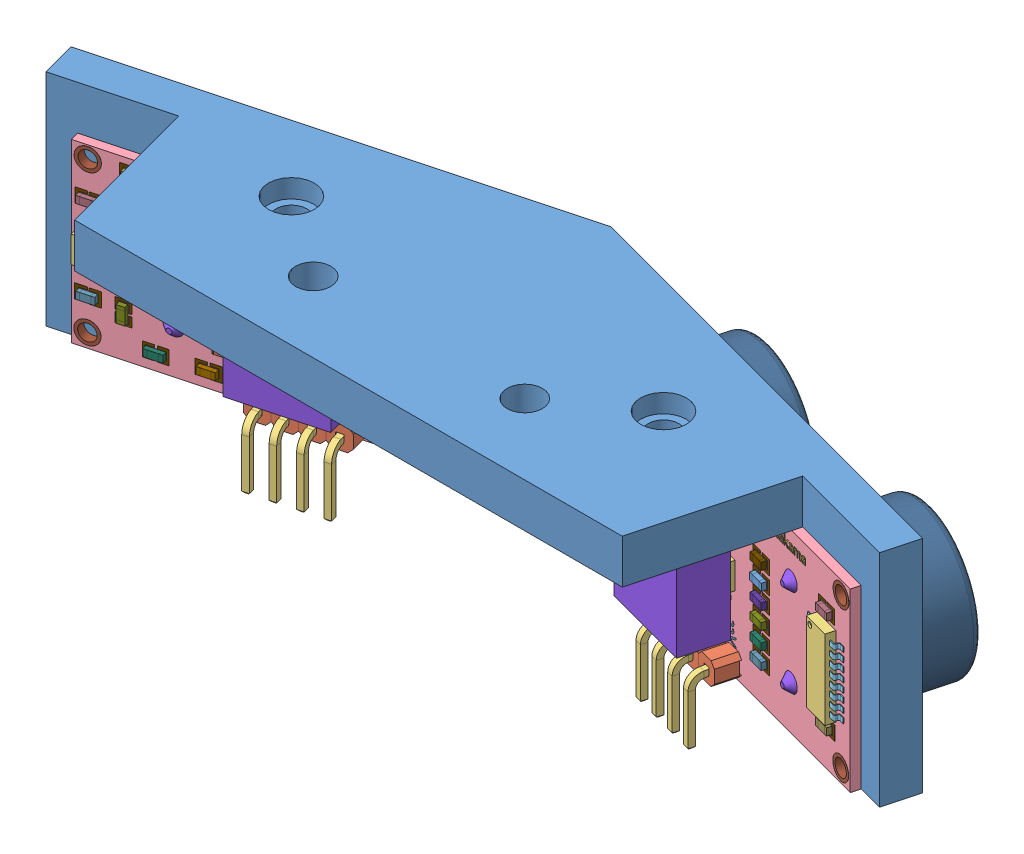
SolidWorks assembly cum_mat_sieu_am, configuration Default. Lengths in mm.
Overall size (428.08 57.86 515.26).
125 component instances, 62 part files, 12 mates.
Components (placement in the parent):
- 11.Ga_sieu_am-1: 11.Ga_sieu_am [Default] at (39.1106 32.5638 61.7658) size (96.59 25 29.76)
- 6. HC-04HC-04.stp-1: 6. HC-04HC-04.stp [Default] at (61.5511 42.5638 72.9551) x (-0.965926 0 -0.258819) z (0.258819 0 -0.965926) size (45 25.57 17.46)
  - HC-04Array.stp-1: HC-04Array.stp [Default] at origin size (10.16 2.54 2.54)
  - HC-04Array001.stp-1: HC-04Array001.stp [Default] at (0 0 1) size (8.32 7.52 6.46)
  - HC-04Placa.stp-1: HC-04Placa.stp [Default] at origin size (45 20 1)
  - HC-04Pad003.stp-1: HC-04Pad003.stp [Default] at (0 0 1) size (10.52 3.38 0.2)
  - HC-04Fillet.stp-1: HC-04Fillet.stp [Default] at (0 0 1) size (10.1 2.84 3)
  - HC-04Array002.stp-1: HC-04Array002.stp [Default] at origin size (9.62 2 1)
  - HC-04Array003.stp-1: HC-04Array003.stp [Default] at (0 0 1) size (28 12 0.8)
  - HC-04Fusion.stp-1: HC-04Fusion.stp [Default] at origin size (6 2 1)
  - HC-04Fillet001.stp-1: HC-04Fillet001.stp [Default] at (0 0 1) size (42 16 12)
  - HC-04Pad005.stp-1: HC-04Pad005.stp [Default] at (0 0 1) size (39.16 13 0.2)
  - HC-04Pad006.stp-1: HC-04Pad006.stp [Default] at (0 0 1) size (35.01 9.04 7)
  - HC-04Fusion001.stp-1: HC-04Fusion001.stp [Default] at (0 0 8) size (31 5 1.5)
  - HC-04Clone_of_Fusion002.stp-1: HC-04Clone_of_Fusion002.stp [Default] at (47.2 -5.5 12.6) size (13 13 0.15)
  - HC-04Clone_of_Fusion003.stp-1: HC-04Clone_of_Fusion003.stp [Default] at (21.2 -5.5 12.6) size (13 13 0.15)
  - HC-04Array005.stp-1: HC-04Array005.stp [Default] at origin size (9.62 2 1)
  - HC-04Array002002.stp-1: HC-04Array002002.stp [Default] at (-5.9 0.1 0.15) size (6.57 1.4 0.56)
  - HC-04Clone_of_Array002002.stp-1: HC-04Clone_of_Array002002.stp [Default] at (-23.9 0.1 0.15) size (6.57 1.4 0.56)
  - HC-04Array002003.stp-1: HC-04Array002003.stp [Default] at (-6.05 0 0.15) size (6.57 1.4 0.56)
  - HC-04Clone_of_Array002003.stp-1: HC-04Clone_of_Array002003.stp [Default] at (-24.05 0 0.15) size (6.57 1.4 0.56)
  - HC-04Integrados.stp-1: HC-04Integrados.stp [Default] at origin size (42.14 9 1)
  - HC-04ShapeString.stp-1: HC-04ShapeString.stp [Default] at (-3.2 -7 1.01) x (0 1 0) z (0 0 1) size (2.53 1.13 0.01)
  - HC-04ShapeString001.stp-1: HC-04ShapeString001.stp [Default] at (-0.6 -7 1.01) x (0 1 0) z (0 0 1) size (2.66 1.45 0.01)
  - HC-04ShapeString002.stp-1: HC-04ShapeString002.stp [Default] at (1.9 -7 1.01) x (0 1 0) z (0 0 1) size (3.21 1.16 0.01)
  - HC-04ShapeString003.stp-1: HC-04ShapeString003.stp [Default] at (4.5 -7 1.01) x (0 1 0) z (0 0 1) size (2.71 1.16 0.01)
  - HC-04ShapeString004.stp-1: HC-04ShapeString004.stp [Default] at (-19.5 -9.3 1.01) size (1.84 2.34 0.01)
  - HC-04ShapeString005.stp-1: HC-04ShapeString005.stp [Default] at (17.5 -9.3 1.01) size (1.82 2.34 0.01)
  - HC-04ShapeString006.stp-1: HC-04ShapeString006.stp [Default] at (-3 3.7 1.01) size (5.52 1.41 0.01)
  - HC-04Pad008.stp-1: HC-04Pad008.stp [Default] at (0 0 -0.01) size (44.56 19.6 1.02)
  - HC-04Scale004.stp-1: HC-04Scale004.stp [Default] at (-1.9 -21.5 -1.5) x (0 1 0) z (0 0 1) size (0.8 1.77 0.5)
  - HC-04Scale027.stp-1: HC-04Scale027.stp [Default] at (-1.9 -10.2323 -1.5) x (0 1 0) z (0 0 1) size (0.8 1.77 0.5)
  - HC-04Scale028.stp-1: HC-04Scale028.stp [Default] at (8.5984 -21.5 -1.5) x (0 1 0) z (0 0 1) size (0.8 1.77 0.5)
  - HC-04Scale029.stp-1: HC-04Scale029.stp [Default] at (8.5984 -19.5867 -1.5) x (0 1 0) z (0 0 1) size (0.8 1.77 0.5)
  - HC-04Scale030.stp-1: HC-04Scale030.stp [Default] at (8.5984 -17.5982 -1.5) x (0 1 0) z (0 0 1) size (0.8 1.77 0.5)
  - HC-04Scale031.stp-1: HC-04Scale031.stp [Default] at (8.5984 -15.6427 -1.5) x (0 1 0) z (0 0 1) size (0.8 1.77 0.5)
  - HC-04Scale032.stp-1: HC-04Scale032.stp [Default] at (8.5984 -11.6848 -1.5) x (0 1 0) z (0 0 1) size (0.8 1.77 0.5)
  - HC-04Scale033.stp-1: HC-04Scale033.stp [Default] at (-26.74 -2 -1.5) x (0 1 0) z (0 0 1) size (0.8 1.85 0.5)
  - HC-04Scale034.stp-1: HC-04Scale034.stp [Default] at (24.9371 -21.5 -1.5) x (0 1 0) z (0 0 1) size (0.8 1.77 0.5)
  - HC-04Scale035.stp-1: HC-04Scale035.stp [Default] at (24.9691 -19.5867 -1.5) x (0 1 0) z (0 0 1) size (0.8 1.77 0.5)
  - HC-04Scale036.stp-1: HC-04Scale036.stp [Default] at (24.9742 -17.5982 -1.5) x (0 1 0) z (0 0 1) size (0.8 1.77 0.5)
  - HC-04Scale037.stp-1: HC-04Scale037.stp [Default] at (-10.4013 -2 -1.5) x (0 1 0) z (0 0 1) size (0.8 1.85 0.5)
  - HC-04Scale038.stp-1: HC-04Scale038.stp [Default] at (-10.4013 -3.9266 -1.5) x (0 1 0) z (0 0 1) size (0.8 1.85 0.5)
  - HC-04Scale039.stp-1: HC-04Scale039.stp [Default] at (-10.4013 -0.0734 -1.5) x (0 1 0) z (0 0 1) size (0.8 1.85 0.5)
  - HC-04Scale040.stp-1: HC-04Scale040.stp [Default] at (24.9742 -9.855 -1.5) x (0 1 0) z (0 0 1) size (0.8 1.77 0.5)
  - HC-04Scale041.stp-1: HC-04Scale041.stp [Default] at (26.5673 -24.0564 -1.5) x (0 1 0) z (0 0 1) size (0.8 1.77 0.5)
  - HC-04Scale042.stp-1: HC-04Scale042.stp [Default] at (26.5673 -7.3333 -1.5) x (0 1 0) z (0 0 1) size (0.8 1.77 0.5)
  - HC-04Scale043.stp-1: HC-04Scale043.stp [Default] at (30.1435 -7.3333 -1.5) x (0 1 0) z (0 0 1) size (0.8 1.77 0.5)
  - HC-04Scale044.stp-1: HC-04Scale044.stp [Default] at (33.5459 -7.3333 -1.5) x (0 1 0) z (0 0 1) size (0.8 1.77 0.5)
  - HC-04Scale045.stp-1: HC-04Scale045.stp [Default] at (37.7181 -11.1827 -1.5) x (0 1 0) z (0 0 1) size (0.8 1.77 0.5)
  - HC-04Scale046.stp-1: HC-04Scale046.stp [Default] at (37.7181 -20.5932 -1.5) x (0 1 0) z (0 0 1) size (0.8 1.77 0.5)
  - HC-04Scale047.stp-1: HC-04Scale047.stp [Default] at (-3.9042 -12.3288 -1.5) x (0 1 0) z (0 0 1) size (0.8 1.85 0.5)
  - HC-04Scale048.stp-1: HC-04Scale048.stp [Default] at (13.5402 13.2894 -1.5) size (0.8 1.85 0.5)
  - HC-04Scale049.stp-1: HC-04Scale049.stp [Default] at (13.5402 23.7909 -1.5) size (0.8 1.85 0.5)
  - HC-04Pad009.stp-1: HC-04Pad009.stp [Default] x (1 0 0) z (0 0 -1) size (42.21 18.43 0.01)
  - HC-04ShapeString007.stp-1: HC-04ShapeString007.stp [Default] at (-3.2 -7 -0.1) x (0 1 0) z (0 0 1) size (2.53 1.13 0.01)
  - HC-04ShapeString008.stp-1: HC-04ShapeString008.stp [Default] at (-0.6 -7 -0.1) x (0 1 0) z (0 0 1) size (2.66 1.45 0.01)
  - HC-04ShapeString009.stp-1: HC-04ShapeString009.stp [Default] at (1.9 -7 -0.1) x (0 1 0) z (0 0 1) size (3.21 1.16 0.01)
  - HC-04ShapeString010.stp-1: HC-04ShapeString010.stp [Default] at (4.5 -7 -0.1) x (0 1 0) z (0 0 1) size (2.71 1.16 0.01)
  - HC-04Fusion002.stp-1: HC-04Fusion002.stp [Default] at origin size (5.7 7.57 0.56)
  - HC-04ShapeString011.stp-1: HC-04ShapeString011.stp [Default] at (-17.5 8.4 1.1) size (7.91 1.16 0.01)
  - HC-04ShapeString012.stp-1: HC-04ShapeString012.stp [Default] at (-7.5 8 -0.1) x (-1 0 0) z (0 0 -1) size (7.91 1.16 0.01)
- 6. HC-04HC-04.stp-2: 6. HC-04HC-04.stp [Default] at (16.6702 42.5638 72.9551) x (-0.965926 0 0.258819) z (-0.258819 0 -0.965926) size (45 25.57 17.46)
  - HC-04Array.stp-1: HC-04Array.stp [Default] at origin size (10.16 2.54 2.54)
  - HC-04Array001.stp-1: HC-04Array001.stp [Default] at (0 0 1) size (8.32 7.52 6.46)
  - HC-04Placa.stp-1: HC-04Placa.stp [Default] at origin size (45 20 1)
  - HC-04Pad003.stp-1: HC-04Pad003.stp [Default] at (0 0 1) size (10.52 3.38 0.2)
  - HC-04Fillet.stp-1: HC-04Fillet.stp [Default] at (0 0 1) size (10.1 2.84 3)
  - HC-04Array002.stp-1: HC-04Array002.stp [Default] at origin size (9.62 2 1)
  - HC-04Array003.stp-1: HC-04Array003.stp [Default] at (0 0 1) size (28 12 0.8)
  - HC-04Fusion.stp-1: HC-04Fusion.stp [Default] at origin size (6 2 1)
  - HC-04Fillet001.stp-1: HC-04Fillet001.stp [Default] at (0 0 1) size (42 16 12)
  - HC-04Pad005.stp-1: HC-04Pad005.stp [Default] at (0 0 1) size (39.16 13 0.2)
  - HC-04Pad006.stp-1: HC-04Pad006.stp [Default] at (0 0 1) size (35.01 9.04 7)
  - HC-04Fusion001.stp-1: HC-04Fusion001.stp [Default] at (0 0 8) size (31 5 1.5)
  - HC-04Clone_of_Fusion002.stp-1: HC-04Clone_of_Fusion002.stp [Default] at (47.2 -5.5 12.6) size (13 13 0.15)
  - HC-04Clone_of_Fusion003.stp-1: HC-04Clone_of_Fusion003.stp [Default] at (21.2 -5.5 12.6) size (13 13 0.15)
  - HC-04Array005.stp-1: HC-04Array005.stp [Default] at origin size (9.62 2 1)
  - HC-04Array002002.stp-1: HC-04Array002002.stp [Default] at (-5.9 0.1 0.15) size (6.57 1.4 0.56)
  - HC-04Clone_of_Array002002.stp-1: HC-04Clone_of_Array002002.stp [Default] at (-23.9 0.1 0.15) size (6.57 1.4 0.56)
  - HC-04Array002003.stp-1: HC-04Array002003.stp [Default] at (-6.05 0 0.15) size (6.57 1.4 0.56)
  - HC-04Clone_of_Array002003.stp-1: HC-04Clone_of_Array002003.stp [Default] at (-24.05 0 0.15) size (6.57 1.4 0.56)
  - HC-04Integrados.stp-1: HC-04Integrados.stp [Default] at origin size (42.14 9 1)
  - HC-04ShapeString.stp-1: HC-04ShapeString.stp [Default] at (-3.2 -7 1.01) x (0 1 0) z (0 0 1) size (2.53 1.13 0.01)
  - HC-04ShapeString001.stp-1: HC-04ShapeString001.stp [Default] at (-0.6 -7 1.01) x (0 1 0) z (0 0 1) size (2.66 1.45 0.01)
  - HC-04ShapeString002.stp-1: HC-04ShapeString002.stp [Default] at (1.9 -7 1.01) x (0 1 0) z (0 0 1) size (3.21 1.16 0.01)
  - HC-04ShapeString003.stp-1: HC-04ShapeString003.stp [Default] at (4.5 -7 1.01) x (0 1 0) z (0 0 1) size (2.71 1.16 0.01)
  - HC-04ShapeString004.stp-1: HC-04ShapeString004.stp [Default] at (-19.5 -9.3 1.01) size (1.84 2.34 0.01)
  - HC-04ShapeString005.stp-1: HC-04ShapeString005.stp [Default] at (17.5 -9.3 1.01) size (1.82 2.34 0.01)
  - HC-04ShapeString006.stp-1: HC-04ShapeString006.stp [Default] at (-3 3.7 1.01) size (5.52 1.41 0.01)
  - HC-04Pad008.stp-1: HC-04Pad008.stp [Default] at (0 0 -0.01) size (44.56 19.6 1.02)
  - HC-04Scale004.stp-1: HC-04Scale004.stp [Default] at (-1.9 -21.5 -1.5) x (0 1 0) z (0 0 1) size (0.8 1.77 0.5)
  - HC-04Scale027.stp-1: HC-04Scale027.stp [Default] at (-1.9 -10.2323 -1.5) x (0 1 0) z (0 0 1) size (0.8 1.77 0.5)
  - HC-04Scale028.stp-1: HC-04Scale028.stp [Default] at (8.5984 -21.5 -1.5) x (0 1 0) z (0 0 1) size (0.8 1.77 0.5)
  - HC-04Scale029.stp-1: HC-04Scale029.stp [Default] at (8.5984 -19.5867 -1.5) x (0 1 0) z (0 0 1) size (0.8 1.77 0.5)
  - HC-04Scale030.stp-1: HC-04Scale030.stp [Default] at (8.5984 -17.5982 -1.5) x (0 1 0) z (0 0 1) size (0.8 1.77 0.5)
  - HC-04Scale031.stp-1: HC-04Scale031.stp [Default] at (8.5984 -15.6427 -1.5) x (0 1 0) z (0 0 1) size (0.8 1.77 0.5)
  - HC-04Scale032.stp-1: HC-04Scale032.stp [Default] at (8.5984 -11.6848 -1.5) x (0 1 0) z (0 0 1) size (0.8 1.77 0.5)
  - HC-04Scale033.stp-1: HC-04Scale033.stp [Default] at (-26.74 -2 -1.5) x (0 1 0) z (0 0 1) size (0.8 1.85 0.5)
  - HC-04Scale034.stp-1: HC-04Scale034.stp [Default] at (24.9371 -21.5 -1.5) x (0 1 0) z (0 0 1) size (0.8 1.77 0.5)
  - HC-04Scale035.stp-1: HC-04Scale035.stp [Default] at (24.9691 -19.5867 -1.5) x (0 1 0) z (0 0 1) size (0.8 1.77 0.5)
  - HC-04Scale036.stp-1: HC-04Scale036.stp [Default] at (24.9742 -17.5982 -1.5) x (0 1 0) z (0 0 1) size (0.8 1.77 0.5)
  - HC-04Scale037.stp-1: HC-04Scale037.stp [Default] at (-10.4013 -2 -1.5) x (0 1 0) z (0 0 1) size (0.8 1.85 0.5)
  - HC-04Scale038.stp-1: HC-04Scale038.stp [Default] at (-10.4013 -3.9266 -1.5) x (0 1 0) z (0 0 1) size (0.8 1.85 0.5)
  - HC-04Scale039.stp-1: HC-04Scale039.stp [Default] at (-10.4013 -0.0734 -1.5) x (0 1 0) z (0 0 1) size (0.8 1.85 0.5)
  - HC-04Scale040.stp-1: HC-04Scale040.stp [Default] at (24.9742 -9.855 -1.5) x (0 1 0) z (0 0 1) size (0.8 1.77 0.5)
  - HC-04Scale041.stp-1: HC-04Scale041.stp [Default] at (26.5673 -24.0564 -1.5) x (0 1 0) z (0 0 1) size (0.8 1.77 0.5)
  - HC-04Scale042.stp-1: HC-04Scale042.stp [Default] at (26.5673 -7.3333 -1.5) x (0 1 0) z (0 0 1) size (0.8 1.77 0.5)
  - HC-04Scale043.stp-1: HC-04Scale043.stp [Default] at (30.1435 -7.3333 -1.5) x (0 1 0) z (0 0 1) size (0.8 1.77 0.5)
  - HC-04Scale044.stp-1: HC-04Scale044.stp [Default] at (33.5459 -7.3333 -1.5) x (0 1 0) z (0 0 1) size (0.8 1.77 0.5)
  - HC-04Scale045.stp-1: HC-04Scale045.stp [Default] at (37.7181 -11.1827 -1.5) x (0 1 0) z (0 0 1) size (0.8 1.77 0.5)
  - HC-04Scale046.stp-1: HC-04Scale046.stp [Default] at (37.7181 -20.5932 -1.5) x (0 1 0) z (0 0 1) size (0.8 1.77 0.5)
  - HC-04Scale047.stp-1: HC-04Scale047.stp [Default] at (-3.9042 -12.3288 -1.5) x (0 1 0) z (0 0 1) size (0.8 1.85 0.5)
  - HC-04Scale048.stp-1: HC-04Scale048.stp [Default] at (13.5402 13.2894 -1.5) size (0.8 1.85 0.5)
  - HC-04Scale049.stp-1: HC-04Scale049.stp [Default] at (13.5402 23.7909 -1.5) size (0.8 1.85 0.5)
  - HC-04Pad009.stp-1: HC-04Pad009.stp [Default] x (1 0 0) z (0 0 -1) size (42.21 18.43 0.01)
  - HC-04ShapeString007.stp-1: HC-04ShapeString007.stp [Default] at (-3.2 -7 -0.1) x (0 1 0) z (0 0 1) size (2.53 1.13 0.01)
  - HC-04ShapeString008.stp-1: HC-04ShapeString008.stp [Default] at (-0.6 -7 -0.1) x (0 1 0) z (0 0 1) size (2.66 1.45 0.01)
  - HC-04ShapeString009.stp-1: HC-04ShapeString009.stp [Default] at (1.9 -7 -0.1) x (0 1 0) z (0 0 1) size (3.21 1.16 0.01)
  - HC-04ShapeString010.stp-1: HC-04ShapeString010.stp [Default] at (4.5 -7 -0.1) x (0 1 0) z (0 0 1) size (2.71 1.16 0.01)
  - HC-04Fusion002.stp-1: HC-04Fusion002.stp [Default] at origin size (5.7 7.57 0.56)
  - HC-04ShapeString011.stp-1: HC-04ShapeString011.stp [Default] at (-17.5 8.4 1.1) size (7.91 1.16 0.01)
  - HC-04ShapeString012.stp-1: HC-04ShapeString012.stp [Default] at (-7.5 8 -0.1) x (-1 0 0) z (0 0 -1) size (7.91 1.16 0.01)
- 12.ganh-1: 12.ganh [Default] at (59.9982 46.6638 78.7506) x (0.965926 0 0.258819) z (0 1 0) size (10 5 19)
- 12.ganh-2: 12.ganh [Default] at (18.2231 46.6638 78.7506) x (0.965926 0 -0.258819) z (0 1 0) size (10 5 19)
Mates (geometry in assembly coordinates):
- Coincident1: coincident aligned: plane of 11.Ga_sieu_am-1 through (39.1106 32.5638 61.7658) normal (0 -1 0); plane of 6. HC-04HC-04.stp-1/HC-04Placa.stp-1 through (39.8177 32.5638 67.1317) normal (0 -1 0)
- Coincident2: coincident anti-aligned: plane of 11.Ga_sieu_am-1 through (86.3716 57.5638 78.5705) normal (-0.258819 0 0.965926); plane of 6. HC-04HC-04.stp-1/HC-04Placa.stp-1 through (83.5432 52.5638 77.8126) normal (0.258819 0 -0.965926)
- Distance1: distance = 1 mm: line of 6. HC-04HC-04.stp-1/HC-04Placa.stp-1 through (40.0766 52.5638 66.1657) axis (0 -1 0); line of 11.Ga_sieu_am-1 through (39.1106 52.5638 65.9069) axis (0 -1 0)
- Coincident5: coincident anti-aligned: plane of 11.Ga_sieu_am-1 through (-8.1504 57.5638 78.5705) normal (0.258819 0 0.965926); plane of 6. HC-04HC-04.stp-2/HC-04Placa.stp-1 through (38.1447 52.5638 66.1657) normal (-0.258819 0 -0.965926)
- Coincident6: coincident aligned: plane of 11.Ga_sieu_am-1 through (39.1106 32.5638 61.7658) normal (0 -1 0); plane of 6. HC-04HC-04.stp-2/HC-04Placa.stp-1 through (-5.0631 32.5638 78.7785) normal (0 -1 0)
- Distance2: distance = 1 mm: line of 6. HC-04HC-04.stp-2/HC-04Placa.stp-1 through (38.1447 32.5638 66.1657) axis (0 1 0); line of 11.Ga_sieu_am-1 through (39.1106 52.5638 65.9069) axis (0 -1 0)
- Coincident8: coincident anti-aligned: plane of 11.Ga_sieu_am-1 through (39.1106 52.5638 61.7658) normal (0 -1 0); plane of 12.ganh-1 through (61.2922 52.5638 73.921) normal (0 1 0)
- Coincident9: coincident anti-aligned: plane of 6. HC-04HC-04.stp-1/HC-04Integrados.stp-1 through (65.156 44.0638 74.9563) normal (-0.258819 0 0.965926); plane of 12.ganh-1 through (61.2922 46.6638 73.921) normal (0.258819 0 -0.965926)
- Width1: width anti-aligned: plane of 12.ganh-1 through (66.1219 46.6638 75.2151) normal (0.965926 0 0.258819); plane of 6. HC-04HC-04.stp-1/HC-04Integrados.stp-1 through (56.4626 46.6638 72.6269) normal (-0.965926 0 -0.258819); plane of 12.ganh-1 through (57.4285 44.0638 72.8857) normal (-0.965926 0 -0.258819); plane of 6. HC-04HC-04.stp-1/HC-04Integrados.stp-1 through (65.156 41.0638 74.9563) normal (0.965926 0 0.258819)
- Coincident11: coincident anti-aligned: plane of 11.Ga_sieu_am-1 through (39.1106 52.5638 61.7658) normal (0 -1 0); plane of 12.ganh-2 through (16.929 52.5638 73.921) normal (0 1 0)
- Coincident12: coincident anti-aligned: plane of 6. HC-04HC-04.stp-2/HC-04Integrados.stp-1 through (20.7927 44.0638 72.8857) normal (0.258819 0 0.965926); plane of 12.ganh-2 through (16.929 46.6638 73.921) normal (-0.258819 0 -0.965926)
- Width2: width anti-aligned: plane of 12.ganh-2 through (21.7586 46.6638 72.6269) normal (0.965926 0 -0.258819); plane of 6. HC-04HC-04.stp-2/HC-04Integrados.stp-1 through (12.0994 46.6638 75.2151) normal (-0.965926 0 0.258819); plane of 12.ganh-2 through (13.0653 44.0638 74.9563) normal (-0.965926 0 0.258819); plane of 6. HC-04HC-04.stp-2/HC-04Integrados.stp-1 through (20.7927 41.0638 72.8857) normal (0.965926 0 -0.258819)
